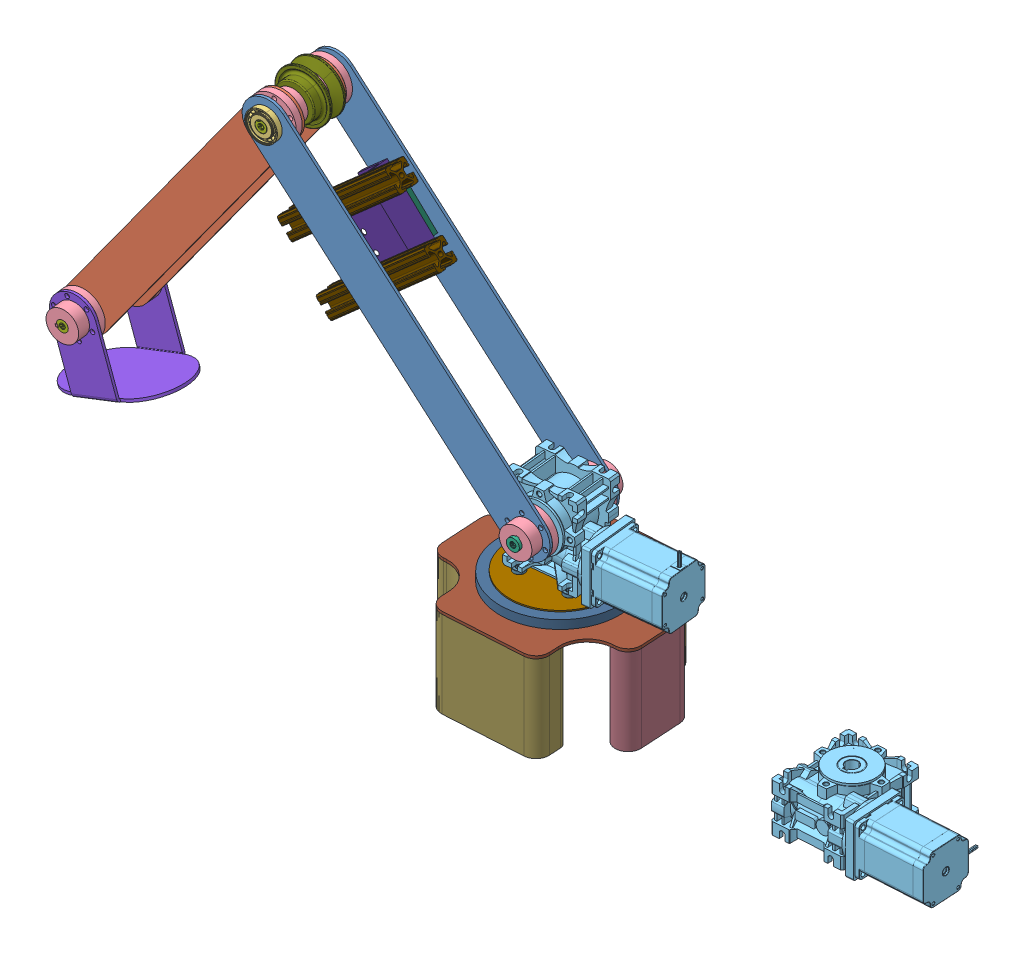
SolidWorks assembly Arm Assembly2, configuration Default. Lengths in mm.
Overall size (1007.94 515.32 219.18).
36 component instances, 19 part files, 85 mates.
Components (placement in the parent):
- Link 2-1: Link 2 [Default] at (47.0194 337.0558 298.1991) x (-0.680313 0.729219 0.073577) z (0.107525 0 0.994202) size (457.2 50.8 3.17)
- Link 3-1: Link 3 [Default] at (-260.6998 630.7223 404.1998) x (-0.575088 -0.815724 0.062197) z (0.107525 0 0.994202) size (406.4 50.8 3.17)
- Flanged Bearing-1: Flanged Bearing [Default] at (-450.225 325.9585 372.0961) x (0.994202 0 -0.107525) z (0.107525 0 0.994202) size (38.1 38.1 12.7)
- Keyed hub-1: Keyed hub [Default] at (37.3262 319.6751 380.8329) x (0.951664 -0.289383 -0.102924) z (-0.287705 -0.957214 0.031116) size (50.8 25.4 50.8)
- Link 2-2: Link 2 [Default] at (56.5945 337.0558 386.7328) x (-0.680313 0.729219 0.073577) z (0.107525 0 0.994202) size (457.2 50.8 3.17)
- Link 3-2: Link 3 [Default] at (-266.6726 630.7223 348.9744) x (-0.575088 -0.815724 0.062197) z (0.107525 0 0.994202) size (406.4 50.8 3.17)
- Flanged Bearing-2: Flanged Bearing [Default] at (-237.9498 616.0299 421.8585) x (-0.946563 0.30584 0.102372) z (0.107525 0 0.994202) size (38.1 38.1 12.7)
- Flanged Bearing-3: Flanged Bearing [Default] at (-444.6101 325.9585 424.0134) x (-0.918373 -0.383049 0.099324) z (-0.107525 0 -0.994202) size (38.1 38.1 12.7)
- Keyed hub-2: Keyed hub [Default] at (-246.9268 616.0299 338.8551) x (0.903538 0.417217 -0.097719) z (0.414798 -0.908807 -0.044861) size (50.8 25.4 50.8)
- Keyed hub-3: Keyed hub [Default] at (29.7995 319.6751 311.2388) x (-0.951664 0.289383 0.102924) z (-0.287705 -0.957214 0.031116) size (50.8 25.4 50.8)
- Keyed hub-4: Keyed hub [Default] at (-238.9057 616.0299 413.02) x (-0.903538 -0.417217 0.097719) z (0.414798 -0.908807 -0.044861) size (50.8 25.4 50.8)
- Flanged Bearing-4: Flanged Bearing [Default] at (-247.8827 616.0299 330.0166) x (0.915497 0.38995 -0.099013) z (-0.107525 0 -0.994202) size (38.1 38.1 12.7)
- Nema Stepper Motor-2: Nema Stepper Motor [Default] at (107.9306 300.7059 337.9928) x (0.994202 0 -0.107525) z (-0.107525 0 -0.994202) size (171.01 100.01 63.01)
- Nema Stepper Motor-3: Nema Stepper Motor [Default] at (426.1519 175.0272 335.1941) x (0.998228 0 -0.059501) z (0 -1 0) size (171.01 100.01 63.01)
- Keyed Drive Shaft-1: Keyed Drive Shaft [Default] at (22.6694 321.928 217.6376) x (0.951664 -0.289383 -0.102924) z (0.107525 0 0.994202) size (19.9 19.9 128.01)
- Keyed Shaft-1: Keyed Shaft [Default] at (-249.5571 616.0299 314.5343) x (0.903538 0.417217 -0.097719) z (0.107525 0 0.994202) size (12.7 12.5 104.14)
- Link 4-1: Link 4 [Default] at (-448.314 244.6162 399.083) x (0.107525 0 0.994202) z (-0.94726 -0.303649 0.102448) size (90.37 102.6 133.86)
- Keyed hub-5: Keyed hub [Default] at (-450.9818 325.9585 365.0987) x (0.301888 -0.952784 -0.03265) z (0.94726 0.303649 -0.102448) size (50.8 25.4 50.8)
- Keyed hub-6: Keyed hub [Default] at (-443.6542 325.9585 432.8518) x (-0.301888 0.952784 0.03265) z (0.94726 0.303649 -0.102448) size (50.8 25.4 50.8)
- Keyed Shaft-2: Keyed Shaft [Default] at (-439.8306 325.9585 468.2056) x (0.301888 -0.952784 -0.03265) z (-0.107525 0 -0.994202) size (12.7 12.5 104.14)
- Bearing maybe-1: Bearing maybe [Default] at (32.1724 257.1751 346.1862) x (0.994202 0 -0.107525) z (0.107525 0 0.994202) size (117.56 1.5 117.56)
- Bearing other part-1: Bearing other part [Default] at (32.1724 247.1751 346.1862) size (140 10 140)
- Top base plate-1: Top base plate [Default] at (33.5723 244.0001 346.2554) x (0.998228 0 -0.059501) z (0.059501 0 0.998228) size (222 3.17 194.94)
- arm base spacer large part-1: arm base spacer large part [Default] at (32.1724 142.4001 346.1862) x (-0.998228 0 0.059501) z (-0.059501 0 -0.998228) size (171.5 101.6 195.24)
- arm base spacer small part-1: arm base spacer small part [Default] at (130.8381 142.4001 364.6329) x (0.998228 0 -0.059501) z (0.059501 0 0.998228) size (30 101.6 78.26)
- 4 mm M6 spacer-1: 4 mm M6 spacer [94669A162] at (62.7675 260.6751 365.0056) x (-1 0 0) z (0 -1 0) size (13 13 4)
- 4 mm M6 spacer-2: 4 mm M6 spacer [94669A162] at (9.0806 260.6751 370.8119) x (1 0 0) z (0 -1 0) size (13 13 4)
- 4 mm M6 spacer-3: 4 mm M6 spacer [94669A162] at (58.0364 260.6751 321.2607) x (1 0 0) z (0 -1 0) size (13 13 4)
- 4 mm M6 spacer-4: 4 mm M6 spacer [94669A162] at (4.3495 260.6751 327.067) x (1 0 0) z (0 -1 0) size (13 13 4)
- 80 kg-1: 80 kg [Default] at (-156.7026 571.7069 383.4867) x (0.650213 -0.756491 -0.070322) z (0.752105 0.654004 -0.081341) size (82 48 30)
- 6204K122_Heavy Duty V-Belt Pulley.step-1: 6204K122_Heavy Duty V-Belt Pulley.step [Default] at (-243.7109 616.0299 368.59) x (0.584363 0.809027 -0.0632) z (0.107525 0 0.994202) size (59.69 59.69 31.75)
- servobracket_80kg-1: servobracket_80kg [Default] at (-150.7716 533.8316 383.6117) x (-0.650213 0.756491 0.070322) z (-0.752105 -0.654004 0.081341) size (87.12 31.24 59.67)
- 47065T553_T-Slotted Framing-1: 47065T553_T-Slotted Framing [47065T553] at (-124.2007 501.2106 393.5121) x (0.107525 0 0.994202) z (-0.752105 -0.654004 0.081341) size (25.4 25.4 152.4)
- 47065T553_T-Slotted Framing-2: 47065T553_T-Slotted Framing [47065T553] at (-165.4277 563.1313 397.9709) x (0.107525 0 0.994202) z (0.752105 0.654004 -0.081341) size (25.4 25.4 152.4)
- 91125A471_Female Threaded Round Standoff-2: 91125A471_Female Threaded Round Standoff [91125A471] at (-116.6227 514.5015 374.0424) x (0.994202 0 -0.107525) z (0.107525 0 0.994202) size (6.35 6.35 38.54)
- 91125A471_Female Threaded Round Standoff-3: 91125A471_Female Threaded Round Standoff [91125A471] at (-165.3886 571.2383 379.3165) x (0.978782 0.175445 -0.105857) z (0.107525 0 0.994202) size (6.35 6.35 38.54)
Mates (geometry in assembly coordinates):
- Concentric3: concentric aligned: cylinder of Keyed hub-1 through (38.1797 319.6751 388.7244) axis (0.107525 0 0.994202) radius 17.4625; cylinder of Link 2-2 through (38.1797 319.6751 388.7244) axis (0.107525 0 0.994202) radius 17.4625
- Coincident2: coincident anti-aligned: plane of Keyed hub-1 through (38.1797 319.6751 388.7244) normal (0.107525 0 0.994202); plane of Link 2-2 through (38.1797 319.6751 388.7244) normal (-0.107525 0 -0.994202)
- Concentric4: concentric aligned: cylinder of Keyed hub-1 through (58.2427 313.5744 386.5546) axis (0.107525 0 0.994202) radius 2.5527; cylinder of Link 2-2 through (58.5841 313.5744 389.7112) axis (0.107525 0 0.994202) radius 2.5527
- Concentric5: concentric anti-aligned: cylinder of Link 2-1 through (28.6046 319.6751 300.1907) axis (0.107525 0 0.994202) radius 17.4625; cylinder of Keyed hub-3 through (28.946 319.6751 303.3473) axis (-0.107525 0 -0.994202) radius 17.4625
- Coincident3: coincident anti-aligned: plane of Link 2-1 through (28.946 319.6751 303.3473) normal (0.107525 0 0.994202); plane of Keyed hub-3 through (28.946 319.6751 303.3473) normal (-0.107525 0 -0.994202)
- Concentric7: concentric anti-aligned: cylinder of Link 2-1 through (13.6617 305.2491 305.0003) axis (0.107525 0 0.994202) radius 2.5527; cylinder of Keyed hub-3 through (13.6617 305.2491 305.0003) axis (-0.107525 0 -0.994202) radius 2.5527
- Concentric8: concentric anti-aligned: cylinder of Keyed hub-1 through (37.3262 319.6751 380.8329) axis (0.107525 0 0.994202) radius 6.35; cylinder of Keyed hub-3 through (29.7995 319.6751 311.2388) axis (-0.107525 0 -0.994202) radius 6.35
- Coincident5: coincident aligned: plane of Keyed hub-1 through (35.8155 320.1345 380.9963) normal (0.951664 -0.289383 -0.102924); plane of Keyed hub-3 through (28.2887 320.1345 311.4022) normal (0.951664 -0.289383 -0.102924)
- Concentric9: concentric aligned: cylinder of Link 2-2 through (-238.2994 616.0299 418.6261) axis (0.107525 0 0.994202) radius 17.4625; cylinder of Flanged Bearing-2 through (-237.267 616.0299 428.1717) axis (0.107525 0 0.994202) radius 17.4625
- Concentric10: concentric anti-aligned: cylinder of Link 2-1 through (-247.8745 616.0299 330.0924) axis (0.107525 0 0.994202) radius 17.4625; cylinder of Flanged Bearing-4 through (-248.5655 616.0299 323.7034) axis (-0.107525 0 -0.994202) radius 17.4625
- Concentric11: concentric anti-aligned: cylinder of Link 3-1 through (-240.1006 616.0299 401.9719) axis (0.107525 0 0.994202) radius 17.4625; cylinder of Keyed hub-4 through (-239.7592 616.0299 405.1285) axis (-0.107525 0 -0.994202) radius 17.4625
- Coincident8: coincident anti-aligned: plane of Link 3-1 through (-239.7592 616.0299 405.1285) normal (0.107525 0 0.994202); plane of Keyed hub-4 through (-239.7592 616.0299 405.1285) normal (-0.107525 0 -0.994202)
- Concentric12: concentric anti-aligned: cylinder of Link 3-1 through (-256.8566 628.2246 406.9776) axis (0.107525 0 0.994202) radius 2.5527; cylinder of Keyed hub-4 through (-256.8566 628.2246 406.9776) axis (-0.107525 0 -0.994202) radius 2.5527
- Concentric13: concentric aligned: cylinder of Link 3-2 through (-246.0733 616.0299 346.7466) axis (0.107525 0 0.994202) radius 17.4625; cylinder of Keyed hub-2 through (-246.0733 616.0299 346.7466) axis (0.107525 0 0.994202) radius 17.4625
- Coincident9: coincident anti-aligned: plane of Link 3-2 through (-246.0733 616.0299 346.7466) normal (-0.107525 0 -0.994202); plane of Keyed hub-2 through (-246.0733 616.0299 346.7466) normal (0.107525 0 0.994202)
- Concentric14: concentric aligned: cylinder of Link 3-2 through (-262.8293 628.2246 351.7523) axis (0.107525 0 0.994202) radius 2.5527; cylinder of Keyed hub-2 through (-263.1707 628.2246 348.5957) axis (0.107525 0 0.994202) radius 2.5527
- Concentric15: concentric anti-aligned: cylinder of Keyed hub-2 through (-246.9268 616.0299 338.8551) axis (0.107525 0 0.994202) radius 6.35; cylinder of Keyed hub-4 through (-238.9057 616.0299 413.02) axis (-0.107525 0 -0.994202) radius 6.35
- Coincident10: coincident aligned: plane of Keyed hub-2 through (-245.4924 616.6922 338.7) normal (-0.903538 -0.417217 0.097719); plane of Keyed hub-4 through (-237.4713 616.6922 412.8649) normal (-0.903538 -0.417217 0.097719)
- Concentric16: concentric aligned: cylinder of Flanged Bearing-2 through (-237.267 616.0299 428.1717) axis (0.107525 0 0.994202) radius 6.35; cylinder of Keyed hub-2 through (-246.9268 616.0299 338.8551) axis (0.107525 0 0.994202) radius 6.35
- Concentric17: concentric aligned: cylinder of Flanged Bearing-1 through (-449.5422 325.9585 378.4093) axis (0.107525 0 0.994202) radius 17.4625; cylinder of Link 3-2 through (-450.5746 325.9585 368.8638) axis (0.107525 0 0.994202) radius 17.4625
- Coincident13: coincident anti-aligned: plane of Flanged Bearing-1 through (-450.5746 343.421 368.8638) normal (0.107525 0 0.994202); plane of Link 3-2 through (-246.0733 616.0299 346.7466) normal (-0.107525 0 -0.994202)
- Concentric18: concentric anti-aligned: cylinder of Link 3-1 through (-444.6019 325.9585 424.0891) axis (0.107525 0 0.994202) radius 17.4625; cylinder of Flanged Bearing-3 through (-445.2929 325.9585 417.7002) axis (-0.107525 0 -0.994202) radius 17.4625
- Coincident14: coincident anti-aligned: plane of Link 3-1 through (-239.7592 616.0299 405.1285) normal (0.107525 0 0.994202); plane of Flanged Bearing-3 through (-450.9107 342.0891 427.9649) normal (-0.107525 0 -0.994202)
- Concentric21: concentric anti-aligned: cylinder of Keyed hub-1 through (37.3262 319.6751 380.8329) axis (0.107525 0 0.994202) radius 6.35; cylinder of Keyed Drive Shaft-1 through (40.4444 319.6751 409.6648) axis (-0.107525 0 -0.994202) radius 7
- Parallel1: parallel anti-aligned: plane of Keyed hub-1 through (35.8155 320.1345 380.9963) normal (0.951664 -0.289383 -0.102924); plane of Keyed Drive Shaft-1 through (32.7085 325.4718 346.1282) normal (-0.951664 0.289383 0.102924)
- Coincident18: coincident anti-aligned: plane of Keyed hub-3 through (29.7995 319.6751 311.2388) normal (0.107525 0 0.994202); plane of Keyed Drive Shaft-1 through (30.5832 326.4293 311.154) normal (-0.107525 0 -0.994202)
- Coincident19: coincident anti-aligned: plane of Keyed hub-1 through (37.3262 319.6751 380.8329) normal (-0.107525 0 -0.994202); plane of Keyed Drive Shaft-1 through (38.1099 326.4293 380.7482) normal (0.107525 0 0.994202)
- Concentric22: concentric anti-aligned: cylinder of Keyed hub-2 through (-246.9268 616.0299 338.8551) axis (0.107525 0 0.994202) radius 6.35; cylinder of Keyed Shaft-1 through (-237.267 616.0299 428.1717) axis (-0.107525 0 -0.994202) radius 6.35
- Coincident20: coincident aligned: plane of Keyed hub-2 through (-245.4924 616.6922 338.7) normal (-0.903538 -0.417217 0.097719); plane of Keyed Shaft-1 through (-237.8029 621.0089 428.2296) normal (-0.903538 -0.417217 0.097719)
- Coincident22: coincident anti-aligned: plane of Link 2-1 through (28.946 319.6751 303.3473) normal (0.107525 0 0.994202); plane of Flanged Bearing-4 through (-240.7631 599.9498 332.5168) normal (-0.107525 0 -0.994202)
- Distance1: distance = 2.54 mm anti-aligned: plane of Flanged Bearing-4 through (-242.7391 605.4346 335.8474) normal (0.107525 0 0.994202); plane of Keyed hub-2 through (-246.9268 616.0299 338.8551) normal (-0.107525 0 -0.994202)
- Coincident24: coincident anti-aligned: plane of Link 2-2 through (38.1797 319.6751 388.7244) normal (-0.107525 0 -0.994202); plane of Flanged Bearing-2 through (-243.6092 599.4042 419.2004) normal (0.107525 0 0.994202)
- Distance2: distance = 2.54 mm anti-aligned: plane of Keyed hub-4 through (-238.9057 616.0299 413.02) normal (0.107525 0 0.994202); plane of Flanged Bearing-2 through (-242.1312 605.075 415.9237) normal (-0.107525 0 -0.994202)
- Coincident26: coincident aligned: plane of Flanged Bearing-2 through (-239.1979 609.9842 428.3805) normal (0.107525 0 0.994202); plane of Keyed Shaft-1 through (-237.267 616.0299 428.1717) normal (0.107525 0 0.994202)
- Concentric23: concentric anti-aligned: cylinder of Link 4-1 through (-442.4593 325.9585 443.8999) axis (-0.107525 0 -0.994202) radius 17.4625; cylinder of Keyed hub-6 through (-442.8007 325.9585 440.7433) axis (0.107525 0 0.994202) radius 17.4625
- Concentric24: concentric anti-aligned: cylinder of Link 4-1 through (-463.2776 330.4579 442.9579) axis (-0.107525 0 -0.994202) radius 2.5527; cylinder of Keyed hub-6 through (-463.2776 330.4579 442.9579) axis (0.107525 0 0.994202) radius 2.5527
- Coincident27: coincident anti-aligned: plane of Link 4-1 through (-431.415 205.5386 439.5119) normal (-0.107525 0 -0.994202); plane of Keyed hub-6 through (-442.8007 325.9585 440.7433) normal (0.107525 0 0.994202)
- Concentric25: concentric anti-aligned: cylinder of Link 4-1 through (-452.1767 325.9585 354.0506) axis (0.107525 0 0.994202) radius 17.4625; cylinder of Keyed hub-5 through (-451.8353 325.9585 357.2072) axis (-0.107525 0 -0.994202) radius 17.4625
- Concentric26: concentric anti-aligned: cylinder of Link 4-1 through (-472.3121 330.4579 359.4218) axis (0.107525 0 0.994202) radius 2.5527; cylinder of Keyed hub-5 through (-472.3121 330.4579 359.4218) axis (-0.107525 0 -0.994202) radius 2.5527
- Concentric27: concentric anti-aligned: cylinder of Keyed hub-5 through (-450.9818 325.9585 365.0987) axis (-0.107525 0 -0.994202) radius 6.35; cylinder of Keyed Shaft-2 through (-452.1207 325.9585 354.5683) axis (0.107525 0 0.994202) radius 6.35
- Coincident31: coincident aligned: plane of Keyed hub-5 through (-451.4611 327.4711 365.1505) normal (0.301888 -0.952784 -0.03265); plane of Keyed Shaft-2 through (-457.0992 326.0288 355.1068) normal (0.301888 -0.952784 -0.03265)
- Coincident32: coincident aligned: plane of Keyed hub-6 through (-440.9231 325.9585 458.1046) normal (0.107525 0 0.994202); plane of Keyed Shaft-2 through (-440.9231 325.9585 458.1046) normal (0.107525 0 0.994202)
- Coincident34: coincident anti-aligned: plane of Link 4-1 through (-440.4496 205.5386 355.9758) normal (0.107525 0 0.994202); plane of Keyed hub-5 through (-451.8353 325.9585 357.2072) normal (-0.107525 0 -0.994202)
- Coincident36: coincident aligned: plane of Keyed hub-6 through (-443.1749 324.446 432.8) normal (-0.301888 0.952784 0.03265); plane of Keyed Shaft-2 through (-456.1407 323.0037 355.0031) normal (-0.301888 0.952784 0.03265)
- Concentric28: concentric anti-aligned: cone of Flanged Bearing-3 through (-443.9993 325.9585 429.6608) axis (-0.107525 0 -0.994202); cylinder of Keyed Shaft-2 through (-452.1207 325.9585 354.5683) axis (0.107525 0 0.994202) radius 6.35
- Distance3: distance = 2.54 mm anti-aligned: plane of Flanged Bearing-3 through (-448.3092 336.5871 430.8004) normal (0.107525 0 0.994202); plane of Keyed hub-6 through (-443.6542 325.9585 432.8518) normal (-0.107525 0 -0.994202)
- Coincident37: coincident anti-aligned: plane of Bearing maybe-1 through (32.1724 257.1751 346.1862) normal (0 -1 0); plane of Bearing other part-1 through (32.1724 257.1751 346.1862) normal (0 1 0)
- Concentric29: concentric aligned: cylinder of Bearing maybe-1 through (32.1724 258.6751 346.1862) axis (0 -1 0) radius 58.7822; cylinder of Bearing other part-1 through (32.1724 257.1751 346.1862) axis (0 -1 0) radius 70
- Coincident38: coincident anti-aligned: plane of Top base plate-1 through (74.0847 244.0001 261.2257) normal (0 -1 0); plane of arm base spacer small part-1 through (130.8381 244.0001 364.6329) normal (0 1 0)
- Coincident40: coincident anti-aligned: plane of Top base plate-1 through (74.0847 244.0001 261.2257) normal (0 -1 0); plane of arm base spacer large part-1 through (32.1724 244.0001 346.1862) normal (0 1 0)
- Coincident45: coincident anti-aligned: plane of Bearing other part-1 through (32.1724 247.1751 346.1862) normal (0 -1 0); plane of Top base plate-1 through (74.0847 247.1751 261.2257) normal (0 1 0)
- Concentric32: concentric aligned: cylinder of Bearing other part-1 through (32.1724 257.1751 346.1862) axis (0 -1 0) radius 70; circle of arm base spacer large part-1
- Coincident50: coincident anti-aligned: plane of Bearing maybe-1 through (32.1724 258.6751 346.1862) normal (0 1 0); plane of 4 mm M6 spacer-3 through (58.0364 258.6751 321.2607) normal (0 -1 0)
- Coincident55: coincident anti-aligned: plane of Nema Stepper Motor-2 through (107.9306 300.7059 337.9928) normal (-0.107525 0 -0.994202); plane of Bearing maybe-1 through (32.1724 257.1751 346.1862) normal (0.107525 0 0.994202)
- Distance5: distance = 76.2 mm aligned: plane of Nema Stepper Motor-2 through (107.9306 300.7059 337.9928) normal (0.994202 0 -0.107525); plane of Bearing maybe-1 through (32.1724 257.1751 346.1862) normal (0.994202 0 -0.107525)
- Coincident57: coincident aligned: plane of Top base plate-1 through (-6.0476 247.1751 446.2586) normal (0.059501 0 0.998228); plane of arm base spacer large part-1 through (84.7912 244.0001 440.844) normal (0.059501 0 0.998228)
- Coincident58: coincident aligned: plane of Top base plate-1 through (-75.7951 247.1751 376.9496) normal (-0.998228 0 0.059501); plane of arm base spacer large part-1 through (-75.8042 244.0001 376.7975) normal (-0.998228 0 0.059501)
- Concentric37: concentric aligned: cylinder of Top base plate-1 through (130.8381 247.1751 364.6329) axis (0 -1 0) radius 15; cylinder of arm base spacer small part-1 through (130.8381 244.0001 364.6329) axis (0 -1 0) radius 15
- Coincident59: coincident aligned: plane of Top base plate-1 through (145.8116 247.1751 363.7404) normal (0.998228 0 -0.059501); plane of arm base spacer small part-1 through (145.8116 244.0001 363.7404) normal (0.998228 0 -0.059501)
- Parallel2: parallel aligned: plane of Nema Stepper Motor-3 through (350.3499 203.0272 320.7095) normal (0 1 0); plane of Top base plate-1 through (74.0847 247.1751 261.2257) normal (0 1 0)
- Parallel3: parallel anti-aligned: plane of Nema Stepper Motor-3 through (312.2058 175.0272 353.0364) normal (-0.998228 0 0.059501); plane of arm base spacer small part-1 through (145.8116 244.0001 363.7404) normal (0.998228 0 -0.059501)
- Coincident61: coincident anti-aligned: plane of Nema Stepper Motor-2 through (76.3373 262.6751 369.573) normal (0 -1 0); plane of 4 mm M6 spacer-1 through (62.7675 262.6751 365.0056) normal (0 1 0)
- Concentric39: concentric aligned: cylinder of Nema Stepper Motor-2 through (62.7675 359.6751 365.0056) axis (0 -1 0) radius 3.25; cylinder of 4 mm M6 spacer-1 through (62.7675 262.6751 365.0056) axis (0 -1 0) radius 3.15
- Coincident62: coincident anti-aligned: plane of Bearing maybe-1 through (32.1724 258.6751 346.1862) normal (0 1 0); plane of 4 mm M6 spacer-1 through (62.7675 258.6751 365.0056) normal (0 -1 0)
- Concentric40: concentric aligned: cylinder of Nema Stepper Motor-2 through (58.0364 359.6751 321.2607) axis (0 -1 0) radius 3.25; cylinder of 4 mm M6 spacer-3 through (58.0364 262.6751 321.2607) axis (0 -1 0) radius 3.15
- Concentric41: concentric aligned: cylinder of Nema Stepper Motor-2 through (4.3495 359.6751 327.067) axis (0 -1 0) radius 3.25; cylinder of 4 mm M6 spacer-4 through (4.3495 262.6751 327.067) axis (0 -1 0) radius 3.15
- Concentric42: concentric aligned: cylinder of Nema Stepper Motor-2 through (9.0806 359.6751 370.8119) axis (0 -1 0) radius 3.25; cylinder of 4 mm M6 spacer-2 through (9.0806 262.6751 370.8119) axis (0 -1 0) radius 3.15
- Concentric43: concentric aligned: cylinder of Keyed hub-1 through (38.1797 319.6751 388.7244) axis (0.107525 0 0.994202) radius 17.4625; cylinder of Nema Stepper Motor-2 through (23.5926 319.6751 253.848) axis (0.107525 0 0.994202) radius 7
- Coincident65: coincident anti-aligned: plane of Nema Stepper Motor-2 through (36.9455 319.6751 377.3537) normal (0.107525 0 0.994202); plane of Keyed Drive Shaft-1 through (36.9499 319.6751 377.3532) normal (-0.107525 0 -0.994202)
- Concentric44: concentric aligned: cylinder of 80 kg-1 through (-128.8622 503.3834 380.4757) axis (-0.107525 0 -0.994202) radius 3; cylinder of servobracket_80kg-1 through (-128.7803 503.3834 381.2333) axis (-0.107525 0 -0.994202) radius 3
- Coincident77: coincident anti-aligned: circle of 80 kg-1; cylinder of servobracket_80kg-1 through (-115.9945 514.5015 379.8505) axis (-0.107525 0 -0.994202) radius 3
- Concentric45: concentric aligned: cylinder of 80 kg-1 through (-177.6282 560.1202 385.7499) axis (-0.107525 0 -0.994202) radius 3; cylinder of servobracket_80kg-1 through (-177.5462 560.1202 386.5074) axis (-0.107525 0 -0.994202) radius 3
- Concentric46: concentric aligned: cylinder of 80 kg-1 through (-164.8424 571.2383 384.367) axis (-0.107525 0 -0.994202) radius 3; cylinder of servobracket_80kg-1 through (-164.7604 571.2383 385.1246) axis (-0.107525 0 -0.994202) radius 3
- Concentric47: concentric anti-aligned: cylinder of Keyed Shaft-1 through (-237.267 616.0299 428.1717) axis (-0.107525 0 -0.994202) radius 6.35; cylinder of 6204K122_Heavy Duty V-Belt Pulley.step-1 through (-242.0039 616.0299 384.373) axis (0.107525 0 0.994202) radius 7.9375
- Coincident80: coincident anti-aligned: plane of 80 kg-1 through (-156.7026 571.7069 383.4867) normal (0.107525 0 0.994202); plane of servobracket_80kg-1 through (-150.8535 533.8316 382.8541) normal (-0.107525 0 -0.994202)
- Coincident81: coincident anti-aligned: plane of Link 2-2 through (38.1797 319.6751 388.7244) normal (-0.107525 0 -0.994202); plane of 47065T553_T-Slotted Framing-1 through (-177.4209 448.2055 412.042) normal (0.107525 0 0.994202)
- Coincident82: coincident anti-aligned: plane of servobracket_80kg-1 through (-150.7716 533.8316 383.6117) normal (0.107525 0 0.994202); plane of 47065T553_T-Slotted Framing-1 through (-185.6013 454.5454 387.3786) normal (-0.107525 0 -0.994202)
- Parallel5: parallel anti-aligned: line of servobracket_80kg-1 through (-103.3442 517.4898 378.4824) axis (-0.752105 -0.654004 0.081341); line of 47065T553_T-Slotted Framing-1 through (-176.5021 443.959 386.3945) axis (0.752105 0.654004 -0.081341)
- Coincident85: coincident anti-aligned: plane of Link 2-2 through (38.1797 319.6751 388.7244) normal (-0.107525 0 -0.994202); plane of 47065T553_T-Slotted Framing-2 through (-109.4764 616.1364 404.6937) normal (0.107525 0 0.994202)
- Coincident86: coincident anti-aligned: plane of servobracket_80kg-1 through (-150.7716 533.8316 383.6117) normal (0.107525 0 0.994202); plane of 47065T553_T-Slotted Framing-2 through (-106.7583 609.7964 378.8516) normal (-0.107525 0 -0.994202)
- Parallel6: parallel anti-aligned: line of servobracket_80kg-1 through (-198.1989 550.1733 388.7411) axis (0.752105 0.654004 -0.081341); line of 47065T553_T-Slotted Framing-2 through (-115.8574 620.3828 379.8357) axis (-0.752105 -0.654004 0.081341)
- Concentric51: concentric anti-aligned: cylinder of servobracket_80kg-1 through (-115.9945 514.5015 379.8505) axis (-0.107525 0 -0.994202) radius 3; cone of 91125A471_Female Threaded Round Standoff-2 through (-118.671 514.5015 355.1028) axis (0.107525 0 0.994202)
- Coincident87: coincident anti-aligned: plane of servobracket_80kg-1 through (-150.8535 533.8316 382.8541) normal (-0.107525 0 -0.994202); plane of 91125A471_Female Threaded Round Standoff-2 through (-116.0764 514.5015 379.0929) normal (0.107525 0 0.994202)
- Concentric53: concentric anti-aligned: cylinder of servobracket_80kg-1 through (-164.7604 571.2383 385.1246) axis (-0.107525 0 -0.994202) radius 3; cone of 91125A471_Female Threaded Round Standoff-3 through (-167.437 571.2383 360.3769) axis (0.107525 0 0.994202)
- Coincident89: coincident anti-aligned: plane of servobracket_80kg-1 through (-150.8535 533.8316 382.8541) normal (-0.107525 0 -0.994202); plane of 91125A471_Female Threaded Round Standoff-3 through (-164.8424 571.2383 384.367) normal (0.107525 0 0.994202)
